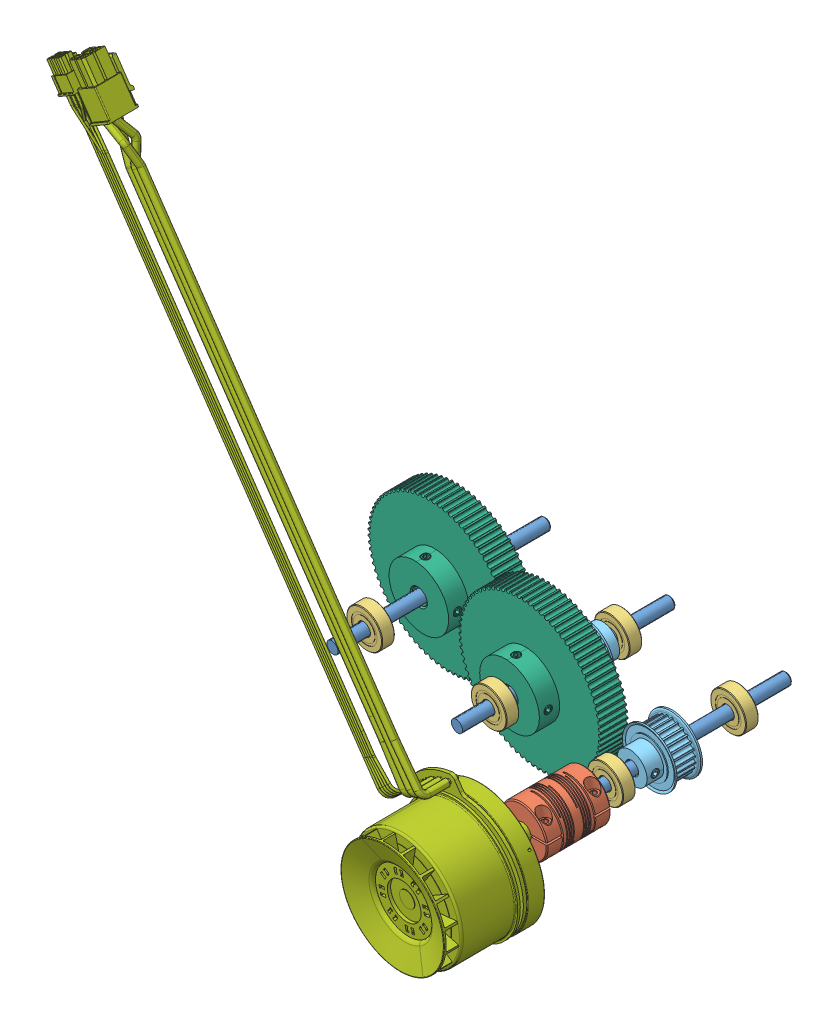
SolidWorks assembly Assembly, configuration Default. Lengths in mm.
Overall size (244.57 335.57 204.23).
16 component instances, 7 part files, 27 mates.
Components (placement in the parent):
- 1482K61_Rotary Shaft-1: 1482K61_Rotary Shaft [1482K61] at (171.5623 109.9965 148.5785) x (0.996996 0.034835 0.069177) z (-0.066525 -0.072256 0.995165) size (6 6 100)
- 2463K6_Clamping Precision Flexible Shaft Coupling-1: 2463K6_Clamping Precision Flexible Shaft Coupling [2463K6] at (171.0076 109.3941 156.8754) x (0.994491 0.076171 0.072011) z (-0.066525 -0.072256 0.995165) size (26.29 26.14 30)
- 6661K11_Ball Bearing-1: 6661K11_Ball Bearing [6661K11] at (176.5844 115.4512 73.452) x (0.996996 0.034835 0.069177) z (-0.066525 -0.072256 0.995165) size (19 19 6)
- 98689A115_General Purpose 18-8 Stainless Steel Washer-1: 98689A115_General Purpose 18-8 Stainless Steel Washer [98689A115] at (112.6968 113.199 96.0002) x (0.997782 -0.002409 0.066525) z (-0.066525 -0.072256 0.995165) size (11 11 1.8)
- 1482K61_Rotary Shaft-2: 1482K61_Rotary Shaft [1482K61] at (109.4611 109.6845 144.4045) x (0.954457 -0.295325 0.042361) z (-0.066525 -0.072256 0.995165) size (6 6 100)
- 1482K61_Rotary Shaft-3: 1482K61_Rotary Shaft [1482K61] at (42.9821 108.0041 139.8384) x (0.997782 -0.002409 0.066525) z (-0.066525 -0.072256 0.995165) size (6 6 100)
- 26toothpulley.stp-1: 26toothpulley.stp [Default] at (113.5484 114.1239 83.2621) x (-0.523948 -0.84627 -0.09647) z (0.066525 0.072256 -0.995165) size (28.1 28.1 20.6)
- 26toothpulley.stp-2: 26toothpulley.stp [Default] at (173.9132 112.55 113.4099) x (-0.032506 -0.996688 -0.074539) z (-0.066525 -0.072256 0.995165) size (28.1 28.1 20.6)
- 80toothpulley.stp-1: 80toothpulley.stp [Default] at (46.3043 111.6125 90.1404) x (0.997782 -0.002409 0.066525) z (-0.066525 -0.072256 0.995165) size (75.56 75.56 22.2)
- 6661K11_Ball Bearing-2: 6661K11_Ball Bearing [6661K11] at (172.7509 111.2875 130.798) x (0.966813 -0.251239 0.046388) z (-0.066525 -0.072256 0.995165) size (19 19 6)
- 6661K11_Ball Bearing-3: 6661K11_Ball Bearing [6661K11] at (114.4832 115.1392 69.2779) x (0.997782 -0.002409 0.066525) z (-0.066525 -0.072256 0.995165) size (19 19 6)
- 6661K11_Ball Bearing-4: 6661K11_Ball Bearing [6661K11] at (110.6497 110.9755 126.624) x (0.990767 0.113299 0.074457) z (-0.066525 -0.072256 0.995165) size (19 19 6)
- 6661K11_Ball Bearing-5: 6661K11_Ball Bearing [6661K11] at (48.0041 113.4588 64.7119) x (0.997782 -0.002409 0.066525) z (-0.066525 -0.072256 0.995165) size (19 19 6)
- 6661K11_Ball Bearing-6: 6661K11_Ball Bearing [6661K11] at (44.1707 109.2951 122.058) x (0.997782 -0.002409 0.066525) z (-0.066525 -0.072256 0.995165) size (19 19 6)
- 80toothpulley.stp-2: 80toothpulley.stp [Default] at (111.7322 112.1513 110.4301) x (0.997782 -0.002409 0.066525) z (-0.066525 -0.072256 0.995165) size (75.56 75.56 22.2)
- EC60fl-200W-V2.stp-1: EC60fl-200W-V2.stp [Default] at (170.453 108.7917 165.1723) x (-0.066525 -0.072256 0.995165) z (0.841923 0.531196 0.09485) size (68.19 353.93 60)
Mates (geometry in assembly coordinates):
- Concentric1: concentric anti-aligned: cylinder of 2463K6_Clamping Precision Flexible Shaft Coupling-1 through (170.0098 108.3102 171.8028) axis (0.066525 0.072256 -0.995165) radius 3; cylinder of EC60fl-200W-V2.stp-1 through (170.6569 109.0131 162.1221) axis (-0.066525 -0.072256 0.995165) radius 4
- Coincident1: coincident aligned: circle of 2463K6_Clamping Precision Flexible Shaft Coupling-1; plane of EC60fl-200W-V2.stp-1 through (170.453 108.7917 165.1723) normal (0.066525 0.072256 -0.995165)
- Concentric3: concentric aligned: cylinder of 1482K61_Rotary Shaft-1 through (164.9097 102.7709 248.095) axis (0.066525 0.072256 -0.995165) radius 3; cylinder of 26toothpulley.stp-2 through (173.3684 111.9582 121.5603) axis (0.066525 0.072256 -0.995165) radius 3
- Concentric4: concentric anti-aligned: cylinder of 1482K61_Rotary Shaft-1 through (164.9097 102.7709 248.095) axis (0.066525 0.072256 -0.995165) radius 3; cylinder of 6661K11_Ball Bearing-2 through (172.5513 111.0707 133.7835) axis (-0.066525 -0.072256 0.995165) radius 3
- Concentric5: concentric anti-aligned: cylinder of 1482K61_Rotary Shaft-1 through (164.9097 102.7709 248.095) axis (0.066525 0.072256 -0.995165) radius 3; cylinder of 6661K11_Ball Bearing-1 through (176.3848 115.2344 76.4375) axis (-0.066525 -0.072256 0.995165) radius 3
- Concentric6: concentric aligned: cylinder of 1482K61_Rotary Shaft-2 through (102.8086 102.4589 243.921) axis (0.066525 0.072256 -0.995165) radius 3; cylinder of 80toothpulley.stp-2 through (111.0686 111.4305 120.3568) axis (0.066525 0.072256 -0.995165) radius 4
- Coincident2: coincident anti-aligned: cylinder of 1482K61_Rotary Shaft-2 through (102.8086 102.4589 243.921) axis (0.066525 0.072256 -0.995165) radius 3; circle of 6661K11_Ball Bearing-4
- Coincident3: coincident anti-aligned: cylinder of 1482K61_Rotary Shaft-2 through (102.8086 102.4589 243.921) axis (0.066525 0.072256 -0.995165) radius 3; circle of 6661K11_Ball Bearing-3
- Concentric7: concentric anti-aligned: cylinder of 1482K61_Rotary Shaft-2 through (102.8086 102.4589 243.921) axis (0.066525 0.072256 -0.995165) radius 3; cylinder of 26toothpulley.stp-1 through (114.0932 114.7156 75.1117) axis (-0.066525 -0.072256 0.995165) radius 3
- Concentric8: concentric aligned: cylinder of 98689A115_General Purpose 18-8 Stainless Steel Washer-1 through (112.5771 113.0689 97.7915) axis (0.066525 0.072256 -0.995165) radius 3.2; cylinder of 1482K61_Rotary Shaft-2 through (102.8086 102.4589 243.921) axis (0.066525 0.072256 -0.995165) radius 3
- Concentric9: concentric anti-aligned: cylinder of 1482K61_Rotary Shaft-3 through (36.3295 100.7785 239.3549) axis (0.066525 0.072256 -0.995165) radius 3; cylinder of 6661K11_Ball Bearing-6 through (43.9711 109.0783 125.0435) axis (-0.066525 -0.072256 0.995165) radius 3
- Concentric10: concentric anti-aligned: cylinder of 1482K61_Rotary Shaft-3 through (36.3295 100.7785 239.3549) axis (0.066525 0.072256 -0.995165) radius 3; cylinder of 6661K11_Ball Bearing-5 through (47.8046 113.242 67.6974) axis (-0.066525 -0.072256 0.995165) radius 3
- Concentric11: concentric aligned: cylinder of 1482K61_Rotary Shaft-3 through (36.3295 100.7785 239.3549) axis (0.066525 0.072256 -0.995165) radius 3; cylinder of 80toothpulley.stp-1 through (45.6407 110.8917 100.0672) axis (0.066525 0.072256 -0.995165) radius 4
- Concentric12: concentric anti-aligned: cylinder of 1482K61_Rotary Shaft-1 through (164.9097 102.7709 248.095) axis (0.066525 0.072256 -0.995165) radius 3; cylinder of 2463K6_Clamping Precision Flexible Shaft Coupling-1 through (172.0055 110.4779 141.9479) axis (-0.066525 -0.072256 0.995165) radius 4
- Coincident5: coincident aligned: plane of 1482K61_Rotary Shaft-1 through (171.5623 109.9965 148.5785) normal (-0.066525 -0.072256 0.995165); circle of 2463K6_Clamping Precision Flexible Shaft Coupling-1
- Parallel2: parallel aligned: plane of 6661K11_Ball Bearing-2 through (174.8207 119.9508 134.58) normal (-0.066525 -0.072256 0.995165); plane of 6661K11_Ball Bearing-4 through (109.3633 119.8753 130.1988) normal (-0.066525 -0.072256 0.995165)
- Parallel3: parallel aligned: plane of 6661K11_Ball Bearing-4 through (109.3633 119.8753 130.1988) normal (-0.066525 -0.072256 0.995165); plane of 6661K11_Ball Bearing-6 through (43.9489 118.2542 125.7082) normal (-0.066525 -0.072256 0.995165)
- Coincident9: coincident anti-aligned: plane of 98689A115_General Purpose 18-8 Stainless Steel Washer-1 through (112.6968 113.199 96.0002) normal (0.066525 0.072256 -0.995165); plane of 26toothpulley.stp-1 through (112.6968 113.199 96.0002) normal (-0.066525 -0.072256 0.995165)
- Coincident10: coincident anti-aligned: circle of 98689A115_General Purpose 18-8 Stainless Steel Washer-1; plane of 80toothpulley.stp-2 through (112.5771 113.0689 97.7915) normal (0.066525 0.072256 -0.995165)
- Coincident11: coincident aligned: plane of 1482K61_Rotary Shaft-1 through (178.2148 117.2221 49.062) normal (0.066525 0.072256 -0.995165); circle of 1482K61_Rotary Shaft-2
- Coincident12: coincident aligned: plane of 6661K11_Ball Bearing-2 through (173.7645 114.6895 128.0982) normal (0.066525 0.072256 -0.995165); plane of 6661K11_Ball Bearing-4 through (110.4594 114.4623 123.8499) normal (0.066525 0.072256 -0.995165)
- Coincident15: coincident aligned: plane of 6661K11_Ball Bearing-4 through (110.4594 114.4623 123.8499) normal (0.066525 0.072256 -0.995165); plane of 6661K11_Ball Bearing-6 through (44.3623 112.8032 119.3109) normal (0.066525 0.072256 -0.995165)
- Coincident16: coincident aligned: plane of 6661K11_Ball Bearing-1 through (176.1595 120.8947 76.8334) normal (-0.066525 -0.072256 0.995165); plane of 6661K11_Ball Bearing-3 through (114.2699 120.5862 72.6737) normal (-0.066525 -0.072256 0.995165)
- Coincident17: coincident aligned: plane of 6661K11_Ball Bearing-3 through (114.2699 120.5862 72.6737) normal (-0.066525 -0.072256 0.995165); circle of 6661K11_Ball Bearing-5
- Coincident18: coincident anti-aligned: plane of 26toothpulley.stp-2 through (174.6783 113.3809 101.9655) normal (-0.066525 -0.072256 0.995165); plane of 80toothpulley.stp-2 through (112.5771 113.0689 97.7915) normal (0.066525 0.072256 -0.995165)
- Coincident19: coincident anti-aligned: plane of 26toothpulley.stp-1 through (112.7833 113.2929 94.7065) normal (0.066525 0.072256 -0.995165); plane of 80toothpulley.stp-1 through (46.3043 111.6125 90.1404) normal (-0.066525 -0.072256 0.995165)
- Coincident20: coincident aligned: plane of 1482K61_Rotary Shaft-2 through (116.1136 116.9101 44.888) normal (0.066525 0.072256 -0.995165); plane of 1482K61_Rotary Shaft-3 through (49.6346 115.2297 40.3219) normal (0.066525 0.072256 -0.995165)
